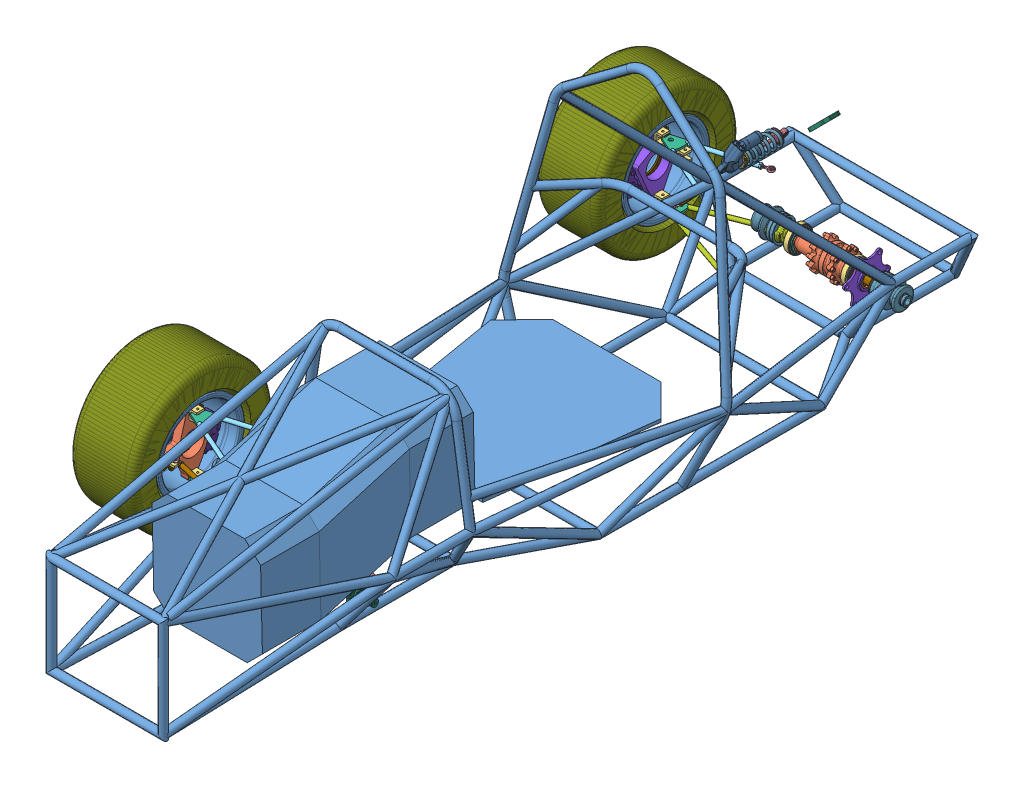
SolidWorks assembly ASSEM_Suspension_RevA, configuration Default. Lengths in mm.
Overall size (1111.1 1095.41 2655.91).
346 component instances, 33 part files, 25 mates.
Components (placement in the parent):
- 2024_Chassis_V1_RevA-1: 2024_Chassis_V1_RevA [Default<As Machined>] at origin size (743.23 992.29 2569.32)
- Differential Assembly-1: Differential Assembly [Default] at (-98.7457 437.9567 -745.2888) x (1 0 0) z (0 -0.960953 -0.276711) size (486.11 199.53 196.01)
  - Drexler Differential-1: Drexler Differential [Default] at (98.7457 177.1174 168.5551) x (0 0.999802 -0.019913) z (0 0.019913 0.999802) size (100 234.25 100)
  - SKF_32010 X-1: SKF_32010 X [Default] at (175.1207 177.1174 168.5551) x (-1 0 0) z (0 -0.454274 -0.890862) size (21.27 80 80)
    - 32010 X_or-1: 32010 X_or [Default] x (1 0 0) z (0 0 -1) size (15.5 80 80)
    - 32010 X_r-1: 32010 X_r [Default] x (1 0 0) z (0 -0.24869 -0.968583) size (15.81 10.45 7.5)
    - 32010 X_r-2: 32010 X_r [Default] x (1 0 0) z (0 -0.481754 -0.876307) size (15.81 10.45 7.5)
    - 32010 X_r-3: 32010 X_r [Default] x (1 0 0) z (0 -0.684547 -0.728969) size (15.81 10.45 7.5)
    - 32010 X_r-4: 32010 X_r [Default] x (1 0 0) z (0 -0.844328 -0.535827) size (15.81 10.45 7.5)
    - 32010 X_r-5: 32010 X_r [Default] x (1 0 0) z (0 -0.951057 -0.309017) size (15.81 10.45 7.5)
    - 32010 X_r-6: 32010 X_r [Default] x (1 0 0) z (0 -0.998027 -0.062791) size (15.81 10.45 7.5)
    - 32010 X_r-7: 32010 X_r [Default] x (1 0 0) z (0 -0.982287 0.187381) size (15.81 10.45 7.5)
    - 32010 X_r-8: 32010 X_r [Default] x (1 0 0) z (0 -0.904827 0.425779) size (15.81 10.45 7.5)
    - 32010 X_r-9: 32010 X_r [Default] x (1 0 0) z (0 -0.770513 0.637424) size (15.81 10.45 7.5)
    - 32010 X_r-10: 32010 X_r [Default] x (1 0 0) z (0 -0.587785 0.809017) size (15.81 10.45 7.5)
    - 32010 X_r-11: 32010 X_r [Default] x (1 0 0) z (0 -0.368125 0.929776) size (15.81 10.45 7.5)
    - 32010 X_r-12: 32010 X_r [Default] x (1 0 0) z (0 -0.125333 0.992115) size (15.81 10.45 7.5)
    - 32010 X_r-13: 32010 X_r [Default] x (1 0 0) z (0 0.125333 0.992115) size (15.81 10.45 7.5)
    - 32010 X_r-14: 32010 X_r [Default] x (1 0 0) z (0 0.368125 0.929776) size (15.81 10.45 7.5)
    - 32010 X_r-15: 32010 X_r [Default] x (1 0 0) z (0 0.587785 0.809017) size (15.81 10.45 7.5)
    - 32010 X_r-16: 32010 X_r [Default] x (1 0 0) z (0 0.770513 0.637424) size (15.81 10.45 7.5)
    - 32010 X_r-17: 32010 X_r [Default] x (1 0 0) z (0 0.904827 0.425779) size (15.81 10.45 7.5)
    - 32010 X_r-18: 32010 X_r [Default] x (1 0 0) z (0 0.982287 0.187381) size (15.81 10.45 7.5)
    - 32010 X_r-19: 32010 X_r [Default] x (1 0 0) z (0 0.998027 -0.062791) size (15.81 10.45 7.5)
    - 32010 X_r-20: 32010 X_r [Default] x (1 0 0) z (0 0.951057 -0.309017) size (15.81 10.45 7.5)
    - 32010 X_r-21: 32010 X_r [Default] x (1 0 0) z (0 0.844328 -0.535827) size (15.81 10.45 7.5)
    - 32010 X_r-22: 32010 X_r [Default] x (1 0 0) z (0 0.684547 -0.728969) size (15.81 10.45 7.5)
    - 32010 X_r-23: 32010 X_r [Default] x (1 0 0) z (0 0.481754 -0.876307) size (15.81 10.45 7.5)
    - 32010 X_r-24: 32010 X_r [Default] x (1 0 0) z (0 0.24869 -0.968583) size (15.81 10.45 7.5)
    - 32010 X_r-25: 32010 X_r [Default] x (1 0 0) z (0 0 -1) size (15.81 10.45 7.5)
    - 32010 X_cage-1: 32010 X_cage [Default] x (1 0 0) z (0 0 -1) size (18.02 76.15 76.15)
    - 32010 X_ir-1: 32010 X_ir [Default] x (1 0 0) z (0 0 -1) size (20 65.95 65.95)
  - SKF_32010 X-2: SKF_32010 X [Default] at (-24.8793 177.1174 168.5551) x (1 0 0) z (0 0.890912 0.454177) size (21.27 80 80)
    - 32010 X_or-1: 32010 X_or [Default] x (1 0 0) z (0 0 -1) size (15.5 80 80)
    - 32010 X_r-1: 32010 X_r [Default] x (1 0 0) z (0 -0.24869 -0.968583) size (15.81 10.45 7.5)
    - 32010 X_r-2: 32010 X_r [Default] x (1 0 0) z (0 -0.481754 -0.876307) size (15.81 10.45 7.5)
    - 32010 X_r-3: 32010 X_r [Default] x (1 0 0) z (0 -0.684547 -0.728969) size (15.81 10.45 7.5)
    - 32010 X_r-4: 32010 X_r [Default] x (1 0 0) z (0 -0.844328 -0.535827) size (15.81 10.45 7.5)
    - 32010 X_r-5: 32010 X_r [Default] x (1 0 0) z (0 -0.951057 -0.309017) size (15.81 10.45 7.5)
    - 32010 X_r-6: 32010 X_r [Default] x (1 0 0) z (0 -0.998027 -0.062791) size (15.81 10.45 7.5)
    - 32010 X_r-7: 32010 X_r [Default] x (1 0 0) z (0 -0.982287 0.187381) size (15.81 10.45 7.5)
    - 32010 X_r-8: 32010 X_r [Default] x (1 0 0) z (0 -0.904827 0.425779) size (15.81 10.45 7.5)
    - 32010 X_r-9: 32010 X_r [Default] x (1 0 0) z (0 -0.770513 0.637424) size (15.81 10.45 7.5)
    - 32010 X_r-10: 32010 X_r [Default] x (1 0 0) z (0 -0.587785 0.809017) size (15.81 10.45 7.5)
    - 32010 X_r-11: 32010 X_r [Default] x (1 0 0) z (0 -0.368125 0.929776) size (15.81 10.45 7.5)
    - 32010 X_r-12: 32010 X_r [Default] x (1 0 0) z (0 -0.125333 0.992115) size (15.81 10.45 7.5)
    - 32010 X_r-13: 32010 X_r [Default] x (1 0 0) z (0 0.125333 0.992115) size (15.81 10.45 7.5)
    - 32010 X_r-14: 32010 X_r [Default] x (1 0 0) z (0 0.368125 0.929776) size (15.81 10.45 7.5)
    - 32010 X_r-15: 32010 X_r [Default] x (1 0 0) z (0 0.587785 0.809017) size (15.81 10.45 7.5)
    - 32010 X_r-16: 32010 X_r [Default] x (1 0 0) z (0 0.770513 0.637424) size (15.81 10.45 7.5)
    - 32010 X_r-17: 32010 X_r [Default] x (1 0 0) z (0 0.904827 0.425779) size (15.81 10.45 7.5)
    - 32010 X_r-18: 32010 X_r [Default] x (1 0 0) z (0 0.982287 0.187381) size (15.81 10.45 7.5)
    - 32010 X_r-19: 32010 X_r [Default] x (1 0 0) z (0 0.998027 -0.062791) size (15.81 10.45 7.5)
    - 32010 X_r-20: 32010 X_r [Default] x (1 0 0) z (0 0.951057 -0.309017) size (15.81 10.45 7.5)
    - 32010 X_r-21: 32010 X_r [Default] x (1 0 0) z (0 0.844328 -0.535827) size (15.81 10.45 7.5)
    - 32010 X_r-22: 32010 X_r [Default] x (1 0 0) z (0 0.684547 -0.728969) size (15.81 10.45 7.5)
    - 32010 X_r-23: 32010 X_r [Default] x (1 0 0) z (0 0.481754 -0.876307) size (15.81 10.45 7.5)
    - 32010 X_r-24: 32010 X_r [Default] x (1 0 0) z (0 0.24869 -0.968583) size (15.81 10.45 7.5)
    - 32010 X_r-25: 32010 X_r [Default] x (1 0 0) z (0 0 -1) size (15.81 10.45 7.5)
    - 32010 X_cage-1: 32010 X_cage [Default] x (1 0 0) z (0 0 -1) size (18.02 76.15 76.15)
    - 32010 X_ir-1: 32010 X_ir [Default] x (1 0 0) z (0 0 -1) size (20 65.95 65.95)
  - D4825 (Drexler Long Tripod Housing)-1: D4825 (Drexler Long Tripod Housing) [Default] at (63.1207 177.1174 168.5551) x (0 0.049326 -0.998783) z (-1 0 0) size (65.36 60.36 166.5)
  - SPIDER_DIFFERENTIAL_ADAPTER-1: SPIDER_DIFFERENTIAL_ADAPTER [Default] at (197.8207 177.0374 168.5892) x (0 -0.59882 0.800884) z (-1 0 0) size (132.58 150 27.1)
  - D4824 (Drexler Medium tripod Housing)-1: D4824 (Drexler Medium tripod Housing) [Default] at (134.3707 177.1174 168.5551) x (0 0.677852 0.735198) z (1 0 0) size (65.36 60.36 155.07)
  - D4672-TA (Tripod)-1: D4672-TA (Tripod) [Default] at (321.1307 160.1151 157.3971) x (1 0 0) z (0 0.676209 0.73671) size (25.48 50.64 55.63)
    - D4672-TA.STEP-1: D4672-TA.STEP [Default] at origin size (25.48 50.64 55.63)
      - FSAE Tripod V2.STEP-1: FSAE Tripod V2.STEP [Default] at (-43.6945 4.946 19.6967) size (24.01 46.11 52.87)
      - FSAE roller_2451.STEP-1: FSAE roller_2451.STEP [Default] at (-43.6945 -7.4365 -1.7504) x (0 0.5 0.866025) z (-1 0 0) size (8.74 25.48 25.48)
      - FSAE roller_2451.STEP-2: FSAE roller_2451.STEP [Default] at (-43.6945 -7.4365 41.1438) x (0 0.5 -0.866025) z (1 0 0) size (8.74 25.48 25.48)
      - FSAE roller_2451.STEP-3: FSAE roller_2451.STEP [Default] at (-43.6945 29.711 19.6967) x (0 -1 0) z (-1 0 0) size (8.74 25.48 25.48)
      - needle.STEP-1: needle.STEP [Default] at (-42.3538 -7.5483 -1.6859) x (1 0 0) z (0 0.5 0.866025) size (1.5 1.5 10.16)
      - needle.STEP-2: needle.STEP [Default] at (-42.3574 -7.2961 -1.8314) x (0.976635 0.186114 -0.107453) z (0 0.5 0.866025) size (1.5 1.5 10.16)
      - needle.STEP-3: needle.STEP [Default] at (-42.4235 -7.0506 -1.9732) x (0.907631 0.363531 -0.209884) z (0 0.5 0.866025) size (1.5 1.5 10.16)
      - needle.STEP-4: needle.STEP [Default] at (-42.5489 -6.823 -2.1046) x (0.796213 0.523959 -0.302508) z (0 0.5 0.866025) size (1.5 1.5 10.16)
      - needle.STEP-5: needle.STEP [Default] at (-42.7279 -6.6242 -2.2194) x (0.647588 0.659903 -0.380995) z (0 0.5 0.866025) size (1.5 1.5 10.16)
      - needle.STEP-6: needle.STEP [Default] at (-42.9521 -6.4632 -2.3123) x (0.468701 0.76501 -0.441678) z (0 0.5 0.866025) size (1.5 1.5 10.16)
      - needle.STEP-7: needle.STEP [Default] at (-43.2109 -6.3478 -2.3789) x (0.267911 0.834367 -0.481722) z (0 0.5 0.866025) size (1.5 1.5 10.16)
      - needle.STEP-8: needle.STEP [Default] at (-43.4924 -6.2833 -2.4162) x (0.054602 0.864733 -0.499254) z (0 0.5 0.866025) size (1.5 1.5 10.16)
      - needle.STEP-9: needle.STEP [Default] at (-43.7833 -6.2726 -2.4224) x (-0.161259 0.854691 -0.493456) z (0 0.5 0.866025) size (1.5 1.5 10.16)
      - needle.STEP-10: needle.STEP [Default] at (-44.07 -6.3163 -2.3971) x (-0.369585 0.804708 -0.464599) z (0 0.5 0.866025) size (1.5 1.5 10.16)
      - needle.STEP-11: needle.STEP [Default] at (-44.3392 -6.4124 -2.3417) x (-0.560639 0.717121 -0.41403) z (0 0.5 0.866025) size (1.5 1.5 10.16)
      - needle.STEP-12: needle.STEP [Default] at (-44.5783 -6.5563 -2.2586) x (-0.725495 0.596023 -0.344114) z (0 0.5 0.866025) size (1.5 1.5 10.16)
      - needle.STEP-13: needle.STEP [Default] at (-44.7761 -6.7413 -2.1517) x (-0.856447 0.447072 -0.258117) z (0 0.5 0.866025) size (1.5 1.5 10.16)
      - needle.STEP-14: needle.STEP [Default] at (-44.9233 -6.9589 -2.0261) x (-0.947378 0.277229 -0.160058) z (0 0.5 0.866025) size (1.5 1.5 10.16)
      - needle.STEP-15: needle.STEP [Default] at (-45.0131 -7.1987 -1.8877) x (-0.994037 0.094432 -0.05452) z (0 0.5 0.866025) size (1.5 1.5 10.16)
      - needle.STEP-16: needle.STEP [Default] at (-45.0413 -7.4497 -1.7428) x (-0.994245 -0.092779 0.053566) z (0 0.5 0.866025) size (1.5 1.5 10.16)
      - needle.STEP-17: needle.STEP [Default] at (-45.0065 -7.7 -1.5982) x (-0.947991 -0.275654 0.159149) z (0 0.5 0.866025) size (1.5 1.5 10.16)
      - needle.STEP-18: needle.STEP [Default] at (-44.9105 -7.9381 -1.4608) x (-0.857437 -0.445647 0.257295) z (0 0.5 0.866025) size (1.5 1.5 10.16)
      - needle.STEP-19: needle.STEP [Default] at (-44.7576 -8.1527 -1.3369) x (-0.726814 -0.594816 0.343417) z (0 0.5 0.866025) size (1.5 1.5 10.16)
      - needle.STEP-20: needle.STEP [Default] at (-44.555 -8.3338 -1.2323) x (-0.562228 -0.716188 0.413491) z (0 0.5 0.866025) size (1.5 1.5 10.16)
      - needle.STEP-21: needle.STEP [Default] at (-44.3122 -8.473 -1.152) x (-0.371368 -0.804092 0.464243) z (0 0.5 0.866025) size (1.5 1.5 10.16)
      - needle.STEP-22: needle.STEP [Default] at (-44.0406 -8.5637 -1.0996) x (-0.163154 -0.854421 0.4933) z (0 0.5 0.866025) size (1.5 1.5 10.16)
      - needle.STEP-23: needle.STEP [Default] at (-43.7528 -8.6018 -1.0776) x (0.052685 -0.864823 0.499306) z (0 0.5 0.866025) size (1.5 1.5 10.16)
      - needle.STEP-24: needle.STEP [Default] at (-43.4622 -8.5854 -1.0871) x (0.266061 -0.834811 0.481978) z (0 0.5 0.866025) size (1.5 1.5 10.16)
      - needle.STEP-25: needle.STEP [Default] at (-43.1825 -8.5153 -1.1275) x (0.467004 -0.765787 0.442128) z (0 0.5 0.866025) size (1.5 1.5 10.16)
      - needle.STEP-26: needle.STEP [Default] at (-42.9268 -8.3949 -1.1971) x (0.646124 -0.660979 0.381616) z (0 0.5 0.866025) size (1.5 1.5 10.16)
      - needle.STEP-27: needle.STEP [Default] at (-42.7069 -8.2296 -1.2925) x (0.79505 -0.525282 0.303272) z (0 0.5 0.866025) size (1.5 1.5 10.16)
      - needle.STEP-28: needle.STEP [Default] at (-42.5332 -8.0272 -1.4093) x (0.906823 -0.365039 0.210755) z (0 0.5 0.866025) size (1.5 1.5 10.16)
      - needle.STEP-29: needle.STEP [Default] at (-42.4137 -7.7973 -1.5421) x (0.97622 -0.187737 0.10839) z (0 0.5 0.866025) size (1.5 1.5 10.16)
      - needle.STEP-30: needle.STEP [Default] at (-42.3538 29.711 19.5676) x (1 0 0) z (0 -1 0) size (1.5 1.5 10.16)
      - needle.STEP-31: needle.STEP [Default] at (-42.3538 -7.3247 41.2084) x (1 0 0) z (0 0.5 -0.866025) size (1.5 1.5 10.16)
      - needle.STEP-32: needle.STEP [Default] at (-42.4137 29.711 19.2801) x (0.97622 0 -0.21678) z (0 -1 0) size (1.5 1.5 10.16)
      - needle.STEP-33: needle.STEP [Default] at (-42.4137 -7.0756 41.3522) x (0.97622 0.187737 0.10839) z (0 0.5 -0.866025) size (1.5 1.5 10.16)
      - needle.STEP-34: needle.STEP [Default] at (-42.5332 29.711 19.0146) x (0.906823 0 -0.421511) z (0 -1 0) size (1.5 1.5 10.16)
      - needle.STEP-35: needle.STEP [Default] at (-42.5332 -6.8457 41.4849) x (0.906823 0.365039 0.210755) z (0 0.5 -0.866025) size (1.5 1.5 10.16)
      - needle.STEP-36: needle.STEP [Default] at (-42.7069 29.711 18.7809) x (0.79505 0 -0.606544) z (0 -1 0) size (1.5 1.5 10.16)
      - needle.STEP-37: needle.STEP [Default] at (-42.7069 -6.6434 41.6017) x (0.79505 0.525282 0.303272) z (0 0.5 -0.866025) size (1.5 1.5 10.16)
      - needle.STEP-38: needle.STEP [Default] at (-42.9268 29.711 18.5901) x (0.646124 0 -0.763232) z (0 -1 0) size (1.5 1.5 10.16)
      - needle.STEP-39: needle.STEP [Default] at (-42.9268 -6.4781 41.6972) x (0.646124 0.660979 0.381616) z (0 0.5 -0.866025) size (1.5 1.5 10.16)
      - needle.STEP-40: needle.STEP [Default] at (-43.1825 29.711 18.4509) x (0.467004 0 -0.884255) z (0 -1 0) size (1.5 1.5 10.16)
      - needle.STEP-41: needle.STEP [Default] at (-43.1825 -6.3576 41.7667) x (0.467004 0.765787 0.442128) z (0 0.5 -0.866025) size (1.5 1.5 10.16)
      - needle.STEP-42: needle.STEP [Default] at (-43.4622 29.711 18.37) x (0.266061 0 -0.963956) z (0 -1 0) size (1.5 1.5 10.16)
      - needle.STEP-43: needle.STEP [Default] at (-43.4622 -6.2875 41.8072) x (0.266061 0.834811 0.481978) z (0 0.5 -0.866025) size (1.5 1.5 10.16)
      - needle.STEP-44: needle.STEP [Default] at (-43.7528 29.711 18.3511) x (0.052685 0 -0.998611) z (0 -1 0) size (1.5 1.5 10.16)
      - needle.STEP-45: needle.STEP [Default] at (-43.7528 -6.2711 41.8166) x (0.052685 0.864823 0.499306) z (0 0.5 -0.866025) size (1.5 1.5 10.16)
      - needle.STEP-46: needle.STEP [Default] at (-44.0406 29.711 18.3951) x (-0.163154 0 -0.986601) z (0 -1 0) size (1.5 1.5 10.16)
      - needle.STEP-47: needle.STEP [Default] at (-44.0406 -6.3092 41.7947) x (-0.163154 0.854421 0.4933) z (0 0.5 -0.866025) size (1.5 1.5 10.16)
      - needle.STEP-48: needle.STEP [Default] at (-44.3122 29.711 18.4999) x (-0.371368 0 -0.928486) z (0 -1 0) size (1.5 1.5 10.16)
      - needle.STEP-49: needle.STEP [Default] at (-44.3122 -6.4 41.7423) x (-0.371368 0.804092 0.464243) z (0 0.5 -0.866025) size (1.5 1.5 10.16)
      - needle.STEP-50: needle.STEP [Default] at (-44.555 29.711 18.6606) x (-0.562228 0 -0.826982) z (0 -1 0) size (1.5 1.5 10.16)
      - needle.STEP-51: needle.STEP [Default] at (-44.555 -6.5392 41.6619) x (-0.562228 0.716188 0.413491) z (0 0.5 -0.866025) size (1.5 1.5 10.16)
      - needle.STEP-52: needle.STEP [Default] at (-44.7576 29.711 18.8697) x (-0.726814 0 -0.686834) z (0 -1 0) size (1.5 1.5 10.16)
      - needle.STEP-53: needle.STEP [Default] at (-44.7576 -6.7203 41.5573) x (-0.726814 0.594816 0.343417) z (0 0.5 -0.866025) size (1.5 1.5 10.16)
      - needle.STEP-54: needle.STEP [Default] at (-44.9105 29.711 19.1175) x (-0.857437 0 -0.514589) z (0 -1 0) size (1.5 1.5 10.16)
      - needle.STEP-55: needle.STEP [Default] at (-44.9105 -6.9349 41.4334) x (-0.857437 0.445647 0.257295) z (0 0.5 -0.866025) size (1.5 1.5 10.16)
      - needle.STEP-56: needle.STEP [Default] at (-45.0065 29.711 19.3924) x (-0.947991 0 -0.318298) z (0 -1 0) size (1.5 1.5 10.16)
      - needle.STEP-57: needle.STEP [Default] at (-45.0065 -7.1729 41.296) x (-0.947991 0.275654 0.159149) z (0 0.5 -0.866025) size (1.5 1.5 10.16)
      - needle.STEP-58: needle.STEP [Default] at (-45.0413 29.711 19.6814) x (-0.994245 0 -0.107132) z (0 -1 0) size (1.5 1.5 10.16)
      - needle.STEP-59: needle.STEP [Default] at (-45.0413 -7.4232 41.1515) x (-0.994245 0.092779 0.053566) z (0 0.5 -0.866025) size (1.5 1.5 10.16)
      - needle.STEP-60: needle.STEP [Default] at (-45.0131 29.711 19.9712) x (-0.994037 0 0.10904) z (0 -1 0) size (1.5 1.5 10.16)
      - needle.STEP-61: needle.STEP [Default] at (-45.0131 -7.6742 41.0066) x (-0.994037 -0.094432 -0.05452) z (0 0.5 -0.866025) size (1.5 1.5 10.16)
      - needle.STEP-62: needle.STEP [Default] at (-44.9233 29.711 20.2482) x (-0.947378 0 0.320117) z (0 -1 0) size (1.5 1.5 10.16)
      - needle.STEP-63: needle.STEP [Default] at (-44.9233 -7.914 40.8681) x (-0.947378 -0.277229 -0.160058) z (0 0.5 -0.866025) size (1.5 1.5 10.16)
      - needle.STEP-64: needle.STEP [Default] at (-44.7761 29.711 20.4994) x (-0.856447 0 0.516234) z (0 -1 0) size (1.5 1.5 10.16)
      - needle.STEP-65: needle.STEP [Default] at (-44.7761 -8.1316 40.7425) x (-0.856447 -0.447072 -0.258117) z (0 0.5 -0.866025) size (1.5 1.5 10.16)
      - needle.STEP-66: needle.STEP [Default] at (-44.5783 29.711 20.7131) x (-0.725495 0 0.688228) z (0 -1 0) size (1.5 1.5 10.16)
      - needle.STEP-67: needle.STEP [Default] at (-44.5783 -8.3166 40.6357) x (-0.725495 -0.596023 -0.344114) z (0 0.5 -0.866025) size (1.5 1.5 10.16)
      - needle.STEP-68: needle.STEP [Default] at (-44.3392 29.711 20.8792) x (-0.560639 0 0.82806) z (0 -1 0) size (1.5 1.5 10.16)
      - needle.STEP-69: needle.STEP [Default] at (-44.3392 -8.4606 40.5526) x (-0.560639 -0.717121 -0.41403) z (0 0.5 -0.866025) size (1.5 1.5 10.16)
      - needle.STEP-70: needle.STEP [Default] at (-44.07 29.711 20.9902) x (-0.369585 0 0.929197) z (0 -1 0) size (1.5 1.5 10.16)
      - needle.STEP-71: needle.STEP [Default] at (-44.07 -8.5566 40.4971) x (-0.369585 -0.804708 -0.464599) z (0 0.5 -0.866025) size (1.5 1.5 10.16)
      - needle.STEP-72: needle.STEP [Default] at (-43.7833 29.711 21.0407) x (-0.161259 0 0.986912) z (0 -1 0) size (1.5 1.5 10.16)
      - needle.STEP-73: needle.STEP [Default] at (-43.7833 -8.6003 40.4719) x (-0.161259 -0.854691 -0.493456) z (0 0.5 -0.866025) size (1.5 1.5 10.16)
      - needle.STEP-74: needle.STEP [Default] at (-43.4924 29.711 21.0283) x (0.054602 0 0.998508) z (0 -1 0) size (1.5 1.5 10.16)
      - needle.STEP-75: needle.STEP [Default] at (-43.4924 -8.5897 40.478) x (0.054602 -0.864733 -0.499254) z (0 0.5 -0.866025) size (1.5 1.5 10.16)
      - needle.STEP-76: needle.STEP [Default] at (-43.2109 29.711 20.9538) x (0.267911 0 0.963444) z (0 -1 0) size (1.5 1.5 10.16)
      - needle.STEP-77: needle.STEP [Default] at (-43.2109 -8.5251 40.5153) x (0.267911 -0.834367 -0.481722) z (0 0.5 -0.866025) size (1.5 1.5 10.16)
      - needle.STEP-78: needle.STEP [Default] at (-42.9521 29.711 20.8205) x (0.468701 0 0.883357) z (0 -1 0) size (1.5 1.5 10.16)
      - needle.STEP-79: needle.STEP [Default] at (-42.9521 -8.4097 40.582) x (0.468701 -0.76501 -0.441678) z (0 0.5 -0.866025) size (1.5 1.5 10.16)
      - needle.STEP-80: needle.STEP [Default] at (-42.7279 29.711 20.6347) x (0.647588 0 0.761991) z (0 -1 0) size (1.5 1.5 10.16)
      - needle.STEP-81: needle.STEP [Default] at (-42.7279 -8.2488 40.6749) x (0.647588 -0.659903 -0.380995) z (0 0.5 -0.866025) size (1.5 1.5 10.16)
      - needle.STEP-82: needle.STEP [Default] at (-42.5489 29.711 20.4051) x (0.796213 0 0.605016) z (0 -1 0) size (1.5 1.5 10.16)
      - needle.STEP-83: needle.STEP [Default] at (-42.5489 -8.0499 40.7897) x (0.796213 -0.523959 -0.302508) z (0 0.5 -0.866025) size (1.5 1.5 10.16)
      - needle.STEP-84: needle.STEP [Default] at (-42.4235 29.711 20.1423) x (0.907631 0 0.419769) z (0 -1 0) size (1.5 1.5 10.16)
      - needle.STEP-85: needle.STEP [Default] at (-42.4235 -7.8224 40.921) x (0.907631 -0.363531 -0.209884) z (0 0.5 -0.866025) size (1.5 1.5 10.16)
      - needle.STEP-86: needle.STEP [Default] at (-42.3574 29.711 19.8588) x (0.976635 0 0.214906) z (0 -1 0) size (1.5 1.5 10.16)
      - needle.STEP-87: needle.STEP [Default] at (-42.3574 -7.5768 41.0628) x (0.976635 -0.186114 -0.107453) z (0 0.5 -0.866025) size (1.5 1.5 10.16)
      - Tripod Retainer.STEP-1: Tripod Retainer.STEP [Default] at (-43.6945 -8.0715 -2.8502) x (0.973299 0.198788 -0.11477) z (0 0.5 0.866025) size (15.88 15.88 1.27)
      - Tripod Retainer.STEP-2: Tripod Retainer.STEP [Default] at (-43.6945 -8.0715 42.2437) x (0.973299 -0.198788 -0.11477) z (0 0.5 -0.866025) size (15.88 15.88 1.27)
      - Tripod Retainer.STEP-3: Tripod Retainer.STEP [Default] at (-43.6945 30.981 19.6967) x (0.973299 0 0.229541) z (0 -1 0) size (15.88 15.88 1.27)
  - D4672-TA (Tripod)-2: D4672-TA (Tripod) [Default] at (-47.6803 161.7899 181.8937) x (1 0 0) z (0 0.890652 -0.454686) size (25.48 50.64 55.63)
    - D4672-TA.STEP-1: D4672-TA.STEP [Default] at origin size (25.48 50.64 55.63)
      - FSAE Tripod V2.STEP-1: FSAE Tripod V2.STEP [Default] at (-43.6945 4.946 19.6967) size (24.01 46.11 52.87)
      - FSAE roller_2451.STEP-1: FSAE roller_2451.STEP [Default] at (-43.6945 -7.4365 -1.7504) x (0 0.5 0.866025) z (-1 0 0) size (8.74 25.48 25.48)
      - FSAE roller_2451.STEP-2: FSAE roller_2451.STEP [Default] at (-43.6945 -7.4365 41.1438) x (0 0.5 -0.866025) z (1 0 0) size (8.74 25.48 25.48)
      - FSAE roller_2451.STEP-3: FSAE roller_2451.STEP [Default] at (-43.6945 29.711 19.6967) x (0 -1 0) z (-1 0 0) size (8.74 25.48 25.48)
      - needle.STEP-1: needle.STEP [Default] at (-42.3538 -7.5483 -1.6859) x (1 0 0) z (0 0.5 0.866025) size (1.5 1.5 10.16)
      - needle.STEP-2: needle.STEP [Default] at (-42.3574 -7.2961 -1.8314) x (0.976635 0.186114 -0.107453) z (0 0.5 0.866025) size (1.5 1.5 10.16)
      - needle.STEP-3: needle.STEP [Default] at (-42.4235 -7.0506 -1.9732) x (0.907631 0.363531 -0.209884) z (0 0.5 0.866025) size (1.5 1.5 10.16)
      - needle.STEP-4: needle.STEP [Default] at (-42.5489 -6.823 -2.1046) x (0.796213 0.523959 -0.302508) z (0 0.5 0.866025) size (1.5 1.5 10.16)
      - needle.STEP-5: needle.STEP [Default] at (-42.7279 -6.6242 -2.2194) x (0.647588 0.659903 -0.380995) z (0 0.5 0.866025) size (1.5 1.5 10.16)
      - needle.STEP-6: needle.STEP [Default] at (-42.9521 -6.4632 -2.3123) x (0.468701 0.76501 -0.441678) z (0 0.5 0.866025) size (1.5 1.5 10.16)
      - needle.STEP-7: needle.STEP [Default] at (-43.2109 -6.3478 -2.3789) x (0.267911 0.834367 -0.481722) z (0 0.5 0.866025) size (1.5 1.5 10.16)
      - needle.STEP-8: needle.STEP [Default] at (-43.4924 -6.2833 -2.4162) x (0.054602 0.864733 -0.499254) z (0 0.5 0.866025) size (1.5 1.5 10.16)
      - needle.STEP-9: needle.STEP [Default] at (-43.7833 -6.2726 -2.4224) x (-0.161259 0.854691 -0.493456) z (0 0.5 0.866025) size (1.5 1.5 10.16)
      - needle.STEP-10: needle.STEP [Default] at (-44.07 -6.3163 -2.3971) x (-0.369585 0.804708 -0.464599) z (0 0.5 0.866025) size (1.5 1.5 10.16)
      - needle.STEP-11: needle.STEP [Default] at (-44.3392 -6.4124 -2.3417) x (-0.560639 0.717121 -0.41403) z (0 0.5 0.866025) size (1.5 1.5 10.16)
      - needle.STEP-12: needle.STEP [Default] at (-44.5783 -6.5563 -2.2586) x (-0.725495 0.596023 -0.344114) z (0 0.5 0.866025) size (1.5 1.5 10.16)
      - needle.STEP-13: needle.STEP [Default] at (-44.7761 -6.7413 -2.1517) x (-0.856447 0.447072 -0.258117) z (0 0.5 0.866025) size (1.5 1.5 10.16)
      - needle.STEP-14: needle.STEP [Default] at (-44.9233 -6.9589 -2.0261) x (-0.947378 0.277229 -0.160058) z (0 0.5 0.866025) size (1.5 1.5 10.16)
      - needle.STEP-15: needle.STEP [Default] at (-45.0131 -7.1987 -1.8877) x (-0.994037 0.094432 -0.05452) z (0 0.5 0.866025) size (1.5 1.5 10.16)
      - needle.STEP-16: needle.STEP [Default] at (-45.0413 -7.4497 -1.7428) x (-0.994245 -0.092779 0.053566) z (0 0.5 0.866025) size (1.5 1.5 10.16)
      - needle.STEP-17: needle.STEP [Default] at (-45.0065 -7.7 -1.5982) x (-0.947991 -0.275654 0.159149) z (0 0.5 0.866025) size (1.5 1.5 10.16)
      - needle.STEP-18: needle.STEP [Default] at (-44.9105 -7.9381 -1.4608) x (-0.857437 -0.445647 0.257295) z (0 0.5 0.866025) size (1.5 1.5 10.16)
      - needle.STEP-19: needle.STEP [Default] at (-44.7576 -8.1527 -1.3369) x (-0.726814 -0.594816 0.343417) z (0 0.5 0.866025) size (1.5 1.5 10.16)
      - needle.STEP-20: needle.STEP [Default] at (-44.555 -8.3338 -1.2323) x (-0.562228 -0.716188 0.413491) z (0 0.5 0.866025) size (1.5 1.5 10.16)
      - needle.STEP-21: needle.STEP [Default] at (-44.3122 -8.473 -1.152) x (-0.371368 -0.804092 0.464243) z (0 0.5 0.866025) size (1.5 1.5 10.16)
      - needle.STEP-22: needle.STEP [Default] at (-44.0406 -8.5637 -1.0996) x (-0.163154 -0.854421 0.4933) z (0 0.5 0.866025) size (1.5 1.5 10.16)
      - needle.STEP-23: needle.STEP [Default] at (-43.7528 -8.6018 -1.0776) x (0.052685 -0.864823 0.499306) z (0 0.5 0.866025) size (1.5 1.5 10.16)
      - needle.STEP-24: needle.STEP [Default] at (-43.4622 -8.5854 -1.0871) x (0.266061 -0.834811 0.481978) z (0 0.5 0.866025) size (1.5 1.5 10.16)
      - needle.STEP-25: needle.STEP [Default] at (-43.1825 -8.5153 -1.1275) x (0.467004 -0.765787 0.442128) z (0 0.5 0.866025) size (1.5 1.5 10.16)
      - needle.STEP-26: needle.STEP [Default] at (-42.9268 -8.3949 -1.1971) x (0.646124 -0.660979 0.381616) z (0 0.5 0.866025) size (1.5 1.5 10.16)
      - needle.STEP-27: needle.STEP [Default] at (-42.7069 -8.2296 -1.2925) x (0.79505 -0.525282 0.303272) z (0 0.5 0.866025) size (1.5 1.5 10.16)
      - needle.STEP-28: needle.STEP [Default] at (-42.5332 -8.0272 -1.4093) x (0.906823 -0.365039 0.210755) z (0 0.5 0.866025) size (1.5 1.5 10.16)
      - needle.STEP-29: needle.STEP [Default] at (-42.4137 -7.7973 -1.5421) x (0.97622 -0.187737 0.10839) z (0 0.5 0.866025) size (1.5 1.5 10.16)
      - needle.STEP-30: needle.STEP [Default] at (-42.3538 29.711 19.5676) x (1 0 0) z (0 -1 0) size (1.5 1.5 10.16)
      - needle.STEP-31: needle.STEP [Default] at (-42.3538 -7.3247 41.2084) x (1 0 0) z (0 0.5 -0.866025) size (1.5 1.5 10.16)
      - needle.STEP-32: needle.STEP [Default] at (-42.4137 29.711 19.2801) x (0.97622 0 -0.21678) z (0 -1 0) size (1.5 1.5 10.16)
      - needle.STEP-33: needle.STEP [Default] at (-42.4137 -7.0756 41.3522) x (0.97622 0.187737 0.10839) z (0 0.5 -0.866025) size (1.5 1.5 10.16)
      - needle.STEP-34: needle.STEP [Default] at (-42.5332 29.711 19.0146) x (0.906823 0 -0.421511) z (0 -1 0) size (1.5 1.5 10.16)
      - needle.STEP-35: needle.STEP [Default] at (-42.5332 -6.8457 41.4849) x (0.906823 0.365039 0.210755) z (0 0.5 -0.866025) size (1.5 1.5 10.16)
      - needle.STEP-36: needle.STEP [Default] at (-42.7069 29.711 18.7809) x (0.79505 0 -0.606544) z (0 -1 0) size (1.5 1.5 10.16)
      - needle.STEP-37: needle.STEP [Default] at (-42.7069 -6.6434 41.6017) x (0.79505 0.525282 0.303272) z (0 0.5 -0.866025) size (1.5 1.5 10.16)
      - needle.STEP-38: needle.STEP [Default] at (-42.9268 29.711 18.5901) x (0.646124 0 -0.763232) z (0 -1 0) size (1.5 1.5 10.16)
      - needle.STEP-39: needle.STEP [Default] at (-42.9268 -6.4781 41.6972) x (0.646124 0.660979 0.381616) z (0 0.5 -0.866025) size (1.5 1.5 10.16)
      - needle.STEP-40: needle.STEP [Default] at (-43.1825 29.711 18.4509) x (0.467004 0 -0.884255) z (0 -1 0) size (1.5 1.5 10.16)
      - needle.STEP-41: needle.STEP [Default] at (-43.1825 -6.3576 41.7667) x (0.467004 0.765787 0.442128) z (0 0.5 -0.866025) size (1.5 1.5 10.16)
      - needle.STEP-42: needle.STEP [Default] at (-43.4622 29.711 18.37) x (0.266061 0 -0.963956) z (0 -1 0) size (1.5 1.5 10.16)
      - needle.STEP-43: needle.STEP [Default] at (-43.4622 -6.2875 41.8072) x (0.266061 0.834811 0.481978) z (0 0.5 -0.866025) size (1.5 1.5 10.16)
      - needle.STEP-44: needle.STEP [Default] at (-43.7528 29.711 18.3511) x (0.052685 0 -0.998611) z (0 -1 0) size (1.5 1.5 10.16)
      - needle.STEP-45: needle.STEP [Default] at (-43.7528 -6.2711 41.8166) x (0.052685 0.864823 0.499306) z (0 0.5 -0.866025) size (1.5 1.5 10.16)
      - needle.STEP-46: needle.STEP [Default] at (-44.0406 29.711 18.3951) x (-0.163154 0 -0.986601) z (0 -1 0) size (1.5 1.5 10.16)
      - needle.STEP-47: needle.STEP [Default] at (-44.0406 -6.3092 41.7947) x (-0.163154 0.854421 0.4933) z (0 0.5 -0.866025) size (1.5 1.5 10.16)
      - needle.STEP-48: needle.STEP [Default] at (-44.3122 29.711 18.4999) x (-0.371368 0 -0.928486) z (0 -1 0) size (1.5 1.5 10.16)
      - needle.STEP-49: needle.STEP [Default] at (-44.3122 -6.4 41.7423) x (-0.371368 0.804092 0.464243) z (0 0.5 -0.866025) size (1.5 1.5 10.16)
      - needle.STEP-50: needle.STEP [Default] at (-44.555 29.711 18.6606) x (-0.562228 0 -0.826982) z (0 -1 0) size (1.5 1.5 10.16)
      - needle.STEP-51: needle.STEP [Default] at (-44.555 -6.5392 41.6619) x (-0.562228 0.716188 0.413491) z (0 0.5 -0.866025) size (1.5 1.5 10.16)
      - needle.STEP-52: needle.STEP [Default] at (-44.7576 29.711 18.8697) x (-0.726814 0 -0.686834) z (0 -1 0) size (1.5 1.5 10.16)
      - needle.STEP-53: needle.STEP [Default] at (-44.7576 -6.7203 41.5573) x (-0.726814 0.594816 0.343417) z (0 0.5 -0.866025) size (1.5 1.5 10.16)
      - needle.STEP-54: needle.STEP [Default] at (-44.9105 29.711 19.1175) x (-0.857437 0 -0.514589) z (0 -1 0) size (1.5 1.5 10.16)
      - needle.STEP-55: needle.STEP [Default] at (-44.9105 -6.9349 41.4334) x (-0.857437 0.445647 0.257295) z (0 0.5 -0.866025) size (1.5 1.5 10.16)
      - needle.STEP-56: needle.STEP [Default] at (-45.0065 29.711 19.3924) x (-0.947991 0 -0.318298) z (0 -1 0) size (1.5 1.5 10.16)
      - needle.STEP-57: needle.STEP [Default] at (-45.0065 -7.1729 41.296) x (-0.947991 0.275654 0.159149) z (0 0.5 -0.866025) size (1.5 1.5 10.16)
      - needle.STEP-58: needle.STEP [Default] at (-45.0413 29.711 19.6814) x (-0.994245 0 -0.107132) z (0 -1 0) size (1.5 1.5 10.16)
      - needle.STEP-59: needle.STEP [Default] at (-45.0413 -7.4232 41.1515) x (-0.994245 0.092779 0.053566) z (0 0.5 -0.866025) size (1.5 1.5 10.16)
      - needle.STEP-60: needle.STEP [Default] at (-45.0131 29.711 19.9712) x (-0.994037 0 0.10904) z (0 -1 0) size (1.5 1.5 10.16)
      - needle.STEP-61: needle.STEP [Default] at (-45.0131 -7.6742 41.0066) x (-0.994037 -0.094432 -0.05452) z (0 0.5 -0.866025) size (1.5 1.5 10.16)
      - needle.STEP-62: needle.STEP [Default] at (-44.9233 29.711 20.2482) x (-0.947378 0 0.320117) z (0 -1 0) size (1.5 1.5 10.16)
      - needle.STEP-63: needle.STEP [Default] at (-44.9233 -7.914 40.8681) x (-0.947378 -0.277229 -0.160058) z (0 0.5 -0.866025) size (1.5 1.5 10.16)
      - needle.STEP-64: needle.STEP [Default] at (-44.7761 29.711 20.4994) x (-0.856447 0 0.516234) z (0 -1 0) size (1.5 1.5 10.16)
      - needle.STEP-65: needle.STEP [Default] at (-44.7761 -8.1316 40.7425) x (-0.856447 -0.447072 -0.258117) z (0 0.5 -0.866025) size (1.5 1.5 10.16)
      - needle.STEP-66: needle.STEP [Default] at (-44.5783 29.711 20.7131) x (-0.725495 0 0.688228) z (0 -1 0) size (1.5 1.5 10.16)
      - needle.STEP-67: needle.STEP [Default] at (-44.5783 -8.3166 40.6357) x (-0.725495 -0.596023 -0.344114) z (0 0.5 -0.866025) size (1.5 1.5 10.16)
      - needle.STEP-68: needle.STEP [Default] at (-44.3392 29.711 20.8792) x (-0.560639 0 0.82806) z (0 -1 0) size (1.5 1.5 10.16)
      - needle.STEP-69: needle.STEP [Default] at (-44.3392 -8.4606 40.5526) x (-0.560639 -0.717121 -0.41403) z (0 0.5 -0.866025) size (1.5 1.5 10.16)
      - needle.STEP-70: needle.STEP [Default] at (-44.07 29.711 20.9902) x (-0.369585 0 0.929197) z (0 -1 0) size (1.5 1.5 10.16)
      - needle.STEP-71: needle.STEP [Default] at (-44.07 -8.5566 40.4971) x (-0.369585 -0.804708 -0.464599) z (0 0.5 -0.866025) size (1.5 1.5 10.16)
      - needle.STEP-72: needle.STEP [Default] at (-43.7833 29.711 21.0407) x (-0.161259 0 0.986912) z (0 -1 0) size (1.5 1.5 10.16)
      - needle.STEP-73: needle.STEP [Default] at (-43.7833 -8.6003 40.4719) x (-0.161259 -0.854691 -0.493456) z (0 0.5 -0.866025) size (1.5 1.5 10.16)
      - needle.STEP-74: needle.STEP [Default] at (-43.4924 29.711 21.0283) x (0.054602 0 0.998508) z (0 -1 0) size (1.5 1.5 10.16)
      - needle.STEP-75: needle.STEP [Default] at (-43.4924 -8.5897 40.478) x (0.054602 -0.864733 -0.499254) z (0 0.5 -0.866025) size (1.5 1.5 10.16)
      - needle.STEP-76: needle.STEP [Default] at (-43.2109 29.711 20.9538) x (0.267911 0 0.963444) z (0 -1 0) size (1.5 1.5 10.16)
      - needle.STEP-77: needle.STEP [Default] at (-43.2109 -8.5251 40.5153) x (0.267911 -0.834367 -0.481722) z (0 0.5 -0.866025) size (1.5 1.5 10.16)
      - needle.STEP-78: needle.STEP [Default] at (-42.9521 29.711 20.8205) x (0.468701 0 0.883357) z (0 -1 0) size (1.5 1.5 10.16)
      - needle.STEP-79: needle.STEP [Default] at (-42.9521 -8.4097 40.582) x (0.468701 -0.76501 -0.441678) z (0 0.5 -0.866025) size (1.5 1.5 10.16)
      - needle.STEP-80: needle.STEP [Default] at (-42.7279 29.711 20.6347) x (0.647588 0 0.761991) z (0 -1 0) size (1.5 1.5 10.16)
      - needle.STEP-81: needle.STEP [Default] at (-42.7279 -8.2488 40.6749) x (0.647588 -0.659903 -0.380995) z (0 0.5 -0.866025) size (1.5 1.5 10.16)
      - needle.STEP-82: needle.STEP [Default] at (-42.5489 29.711 20.4051) x (0.796213 0 0.605016) z (0 -1 0) size (1.5 1.5 10.16)
      - needle.STEP-83: needle.STEP [Default] at (-42.5489 -8.0499 40.7897) x (0.796213 -0.523959 -0.302508) z (0 0.5 -0.866025) size (1.5 1.5 10.16)
      - needle.STEP-84: needle.STEP [Default] at (-42.4235 29.711 20.1423) x (0.907631 0 0.419769) z (0 -1 0) size (1.5 1.5 10.16)
      - needle.STEP-85: needle.STEP [Default] at (-42.4235 -7.8224 40.921) x (0.907631 -0.363531 -0.209884) z (0 0.5 -0.866025) size (1.5 1.5 10.16)
      - needle.STEP-86: needle.STEP [Default] at (-42.3574 29.711 19.8588) x (0.976635 0 0.214906) z (0 -1 0) size (1.5 1.5 10.16)
      - needle.STEP-87: needle.STEP [Default] at (-42.3574 -7.5768 41.0628) x (0.976635 -0.186114 -0.107453) z (0 0.5 -0.866025) size (1.5 1.5 10.16)
      - Tripod Retainer.STEP-1: Tripod Retainer.STEP [Default] at (-43.6945 -8.0715 -2.8502) x (0.973299 0.198788 -0.11477) z (0 0.5 0.866025) size (15.88 15.88 1.27)
      - Tripod Retainer.STEP-2: Tripod Retainer.STEP [Default] at (-43.6945 -8.0715 42.2437) x (0.973299 -0.198788 -0.11477) z (0 0.5 -0.866025) size (15.88 15.88 1.27)
      - Tripod Retainer.STEP-3: Tripod Retainer.STEP [Default] at (-43.6945 30.981 19.6967) x (0.973299 0 0.229541) z (0 -1 0) size (15.88 15.88 1.27)
  - 615-3 (Triangular Tripod Housing Boot)-1: 615-3 (Triangular Tripod Housing Boot) [Default] at (336.0855 177.1174 168.5551) x (0 0.694966 -0.719043) z (1 0 0) size (84.51 84.51 88.49)
  - 615-3 (Triangular Tripod Housing Boot)-2: 615-3 (Triangular Tripod Housing Boot) [Default] at (-150.024 177.1174 168.5551) x (0 -0.881387 -0.472395) z (-1 0 0) size (84.51 84.51 88.49)
- KAZ_Steering_Rack_-_Dumb_Solid-1: KAZ_Steering_Rack_-_Dumb_Solid [Default] at (0 198.8947 1049.6828) x (1 0 0) z (0 1 0) size (386.71 91.39 96.37)
- HoosierTyres_43100Slicks-1: HoosierTyres_43100Slicks [Default] at (-712.47 204.47 902.2716) x (0 -1 0) z (0 0 1) size (459.74 205.74 459.74)
- HoosierTyres_43100Slicks-2: HoosierTyres_43100Slicks [Default] at (-737.87 204.47 -621.7284) x (0 1 0) z (0 0 -1) size (459.74 205.74 459.74)
- ASSEM_Front_WheelUprBrakes-1: ASSEM_Front_WheelUprBrakes [Default] at (-619.125 204.47 902.2716) x (-1 0 0) z (0 0 -1) size (205.74 465.04 465.04)
  - Willwood_Calipers-4: Willwood_Calipers [Default] at (-33.147 7.7199 -7.8202) x (0 0.927952 0.372699) z (1 0 0) size (100.77 53.34 71.25)
  - 7inRotor_Custom-1: 7inRotor_Custom [Default] at (-30.607 0 0) x (0 -0.991825 -0.127604) z (0 0.127604 -0.991825) size (175.34 5.08 177.8)
  - HoosierTyres_43100Slicks-1: HoosierTyres_43100Slicks [Default] at (93.345 0 0) x (0 0.999933 0.011596) z (0 -0.011596 0.999933) size (459.74 205.74 459.74)
  - OZ 10x7 FSAE wheel.stp-1: OZ 10x7 FSAE wheel.stp [Default] at (-9.6203 0 0) x (0 0.669999 -0.742362) z (1 0 0) size (282.17 282.17 189.8)
  - Upright_front-2: Upright_front [Default] at (-51.816 0 0) x (0 0 1) z (-1 0 0) size (170.28 202.6 25.4)
  - UBracket_Upright-1: UBracket_Upright [Default] at (-77.216 71.843 -12.7) x (0 1 0) z (1 0 0) size (31.64 25.4 25.4)
  - UBracket_Upright-2: UBracket_Upright [Default] at (-77.216 -105.3614 -12.7) x (0 1 0) z (1 0 0) size (31.64 25.4 25.4)
  - UBracket_Upright-3: UBracket_Upright [Default] at (-77.216 -15.8222 -84.5631) x (0 1 0) z (1 0 0) size (31.64 25.4 25.4)
- Wishbone_Full-2: Wishbone_Full [Default] at (-559.1993 294.0993 900.1762) x (0.063338 0 -0.997992) z (0.997992 0 0.063338) size (221.1 13.97 268.6)
  - Arm_Weldment1-1: Arm_Weldment1 [Default] at (-39.2885 1.138 55.188) x (-0.939693 0 -0.34202) z (0 1 0) size (19.05 229.31 13.97)
    - 60645K121_Ball Joint Rod End-1: 60645K121_Ball Joint Rod End [60645K121] at (-18.0437 209.4907 -1.138) size (19.05 49.39 9.53)
    - Rod_Wishbone-1: Rod_Wishbone [Default] at (-18.0437 3.9907 -1.138) size (15.98 195.5 13.97)
  - Arm_Weldment1-2: Arm_Weldment1 [Default] at (4.3238 1.138 64.6358) x (-0.939693 0 0.34202) z (0 1 0) size (19.05 229.31 13.97)
    - 60645K121_Ball Joint Rod End-1: 60645K121_Ball Joint Rod End [60645K121] at (-18.0437 209.4907 -1.138) size (19.05 49.39 9.53)
    - Rod_Wishbone-1: Rod_Wishbone [Default] at (-18.0437 3.9907 -1.138) size (15.98 195.5 13.97)
  - Wishbone_Weldment2-1: Wishbone_Weldment2 [Default] at (0.0094 -3.175 33.2314) size (60.81 6.35 56.08)
- FR_Wishbone_Full-1: FR_Wishbone_Full [Default] at (-559.2596 113.415 902.8921) x (-0.018388 0 -0.999831) z (0.999831 0 -0.018388) size (283.72 21.98 364.08)
  - Wishbone_Weldment2-1: Wishbone_Weldment2 [Default] at (0.0094 -3.175 33.2314) size (60.81 6.35 56.08)
  - FR_BottomArm_Weldment1-1: FR_BottomArm_Weldment1 [Default] at (-10.6928 6.9131 82.8687) x (0.794652 0.533737 0.28923) z (0.501549 -0.845651 0.182549) size (19.05 313.21 13.97)
    - 60645K121_Ball Joint Rod End-1: 60645K121_Ball Joint Rod End [60645K121] at (-19.1608 277.8138 -3.9185) size (19.05 49.39 9.53)
    - Rod_Wishbone_B-1: Rod_Wishbone_B [Default] at (-19.1608 -11.5862 -3.9185) size (15.98 284.4 13.97)
  - FR_BottomArm_Weldment1-2: FR_BottomArm_Weldment1 [Default] at (43.952 -9.5492 70.8548) x (0.895366 -0.303509 -0.325887) z (-0.285205 -0.952829 0.103806) size (19.05 313.21 13.97)
    - 60645K121_Ball Joint Rod End-1: 60645K121_Ball Joint Rod End [60645K121] at (-19.1608 277.8138 -3.9185) size (19.05 49.39 9.53)
    - Rod_Wishbone_B-1: Rod_Wishbone_B [Default] at (-19.1608 -11.5862 -3.9185) size (15.98 284.4 13.97)
- ASSEM_Rear_WheelUprBrakes-1: ASSEM_Rear_WheelUprBrakes [Default] at (-644.525 204.47 -621.7284) x (-1 0 0) z (0 0 -1) size (205.74 465.04 465.04)
  - Willwood_Calipers-4: Willwood_Calipers [Default] at (-33.147 7.7179 7.821) x (0 -0.927953 0.372696) z (1 0 0) size (100.77 53.34 71.25)
  - 7inRotor_Custom-1: 7inRotor_Custom [Default] at (-30.607 0 0) x (0 -0.991825 -0.127604) z (0 0.127604 -0.991825) size (175.34 5.08 177.8)
  - HoosierTyres_43100Slicks-1: HoosierTyres_43100Slicks [Default] at (93.345 0 0) x (0 0.999933 0.011596) z (0 -0.011596 0.999933) size (459.74 205.74 459.74)
  - OZ 10x7 FSAE wheel.stp-1: OZ 10x7 FSAE wheel.stp [Default] at (-9.6203 0 0) x (0 0.669999 -0.742362) z (1 0 0) size (282.17 282.17 189.8)
  - UBracket_Upright-1: UBracket_Upright [Default] at (-77.216 71.843 -12.7) x (0 1 0) z (1 0 0) size (31.64 25.4 25.4)
  - UBracket_Upright-2: UBracket_Upright [Default] at (-77.216 -105.3614 -12.7) x (0 1 0) z (1 0 0) size (31.64 25.4 25.4)
  - UBracket_Upright-3: UBracket_Upright [Default] at (-77.216 -15.8222 59.1631) x (0 1 0) z (1 0 0) size (31.64 25.4 25.4)
  - Upright_Rear-2: Upright_Rear [Default] at (-77.216 0 0) x (0 0 -1) z (1 0 0) size (170.28 202.6 25.4)
- FR_Wishbone_Full-2: FR_Wishbone_Full [Default] at (-559.2596 113.415 -621.1079) x (-0.018388 0 -0.999831) z (0.999831 0 -0.018388) size (283.72 21.98 364.08)
  - Wishbone_Weldment2-1: Wishbone_Weldment2 [Default] at (0.0094 -3.175 33.2314) size (60.81 6.35 56.08)
  - FR_BottomArm_Weldment1-1: FR_BottomArm_Weldment1 [Default] at (-10.6928 6.9131 82.8687) x (0.794652 0.533737 0.28923) z (0.501549 -0.845651 0.182549) size (19.05 313.21 13.97)
    - 60645K121_Ball Joint Rod End-1: 60645K121_Ball Joint Rod End [60645K121] at (-19.1608 277.8138 -3.9185) size (19.05 49.39 9.53)
    - Rod_Wishbone_B-1: Rod_Wishbone_B [Default] at (-19.1608 -11.5862 -3.9185) size (15.98 284.4 13.97)
  - FR_BottomArm_Weldment1-2: FR_BottomArm_Weldment1 [Default] at (43.952 -9.5492 70.8548) x (0.895366 -0.303509 -0.325887) z (-0.285205 -0.952829 0.103806) size (19.05 313.21 13.97)
    - 60645K121_Ball Joint Rod End-1: 60645K121_Ball Joint Rod End [60645K121] at (-19.1608 277.8138 -3.9185) size (19.05 49.39 9.53)
    - Rod_Wishbone_B-1: Rod_Wishbone_B [Default] at (-19.1608 -11.5862 -3.9185) size (15.98 284.4 13.97)
- Wishbone_Full-3: Wishbone_Full [Default] at (-559.1993 294.0993 -623.8238) x (0.063338 0 -0.997992) z (0.997992 0 0.063338) size (221.1 13.97 268.6)
  - Arm_Weldment1-1: Arm_Weldment1 [Default] at (-39.2885 1.138 55.188) x (-0.939693 0 -0.34202) z (0 1 0) size (19.05 229.31 13.97)
    - 60645K121_Ball Joint Rod End-1: 60645K121_Ball Joint Rod End [60645K121] at (-18.0437 209.4907 -1.138) size (19.05 49.39 9.53)
    - Rod_Wishbone-1: Rod_Wishbone [Default] at (-18.0437 3.9907 -1.138) size (15.98 195.5 13.97)
  - Arm_Weldment1-2: Arm_Weldment1 [Default] at (4.3238 1.138 64.6358) x (-0.939693 0 0.34202) z (0 1 0) size (19.05 229.31 13.97)
    - 60645K121_Ball Joint Rod End-1: 60645K121_Ball Joint Rod End [60645K121] at (-18.0437 209.4907 -1.138) size (19.05 49.39 9.53)
    - Rod_Wishbone-1: Rod_Wishbone [Default] at (-18.0437 3.9907 -1.138) size (15.98 195.5 13.97)
  - Wishbone_Weldment2-1: Wishbone_Weldment2 [Default] at (0.0094 -3.175 33.2314) size (60.81 6.35 56.08)
- TieRod-1: TieRod [Default] at (-343.9724 201.6783 1005.1556) x (0.223812 0 -0.974632) z (0 1 0) size (19.05 382.22 13.97)
  - RodTubing-1: RodTubing [Default] at (-10.5136 -149.457 1.85) size (15.98 314.8 13.97)
  - 60645K121_Ball Joint Rod End-1: 60645K121_Ball Joint Rod End [60645K121] at (-10.5136 170.0984 1.85) size (19.05 49.39 9.53)
  - 60645K121_Ball Joint Rod End-2: 60645K121_Ball Joint Rod End [60645K121] at (-10.5136 -164.5 1.85) x (-1 0 0) z (0 0 1) size (19.05 49.39 9.53)
- Ohlins TTX25 Shock 50mm-1: Ohlins TTX25 Shock 50mm [Default] at (-302.3187 305.8561 941.9451) x (0.651974 -0.755599 -0.063248) z (-0.063248 -0.137317 0.988506) size (68.2 222.5 95.1)
  - Body-1: Body [Default] at origin size (40.15 132 80.5)
  - M8 ball-1: M8 ball [Default] x (0 0 -1) z (1 0 0) size (12.5 12.5 8)
  - M8 ball-2: M8 ball [Default] at (0 -199.5 0) x (0 0 -1) z (1 0 0) size (12.5 12.5 8)
  - Tightening nut-1: Tightening nut [Default] at (0 -4 0) x (-0.593403 0 0.804906) z (-0.804906 0 -0.593403) size (48.77 20 48.77)
  - Piston-1: Piston [Default] at (0 0.13 0) x (-0.999632 0 -0.027131) z (0.027131 0 -0.999632) size (46 115.5 45.56)
  - Spring-1: Spring [Default] at (0 -176 0) size (54.68 133 54.06)
- Rocker-1: Rocker [Default] at (-147.5 187.7104 976.6436) x (0.804613 0.5938 0) z (0.5938 -0.804613 0) size (63.62 10 93.34)
- Ohlins TTX25 Shock 50mm-2: Ohlins TTX25 Shock 50mm [Default] at (-99.1058 217.885 964.6775) x (0.032629 0.170283 -0.984855) z (0.185343 0.967258 0.173381) size (68.2 222.5 95.1)
  - Body-1: Body [Default] at origin size (40.15 132 80.5)
  - M8 ball-1: M8 ball [Default] x (0 0 -1) z (1 0 0) size (12.5 12.5 8)
  - M8 ball-2: M8 ball [Default] at (0 -199.5 0) x (0 0 -1) z (1 0 0) size (12.5 12.5 8)
  - Tightening nut-1: Tightening nut [Default] at (0 -4 0) x (-0.593403 0 0.804906) z (-0.804906 0 -0.593403) size (48.77 20 48.77)
  - Piston-1: Piston [Default] at (0 0.13 0) x (-0.999632 0 -0.027131) z (0.027131 0 -0.999632) size (46 115.5 45.56)
  - Spring-1: Spring [Default] at (0 -176 0) size (54.68 133 54.06)
- TieRod-2: TieRod [Default] at (-357.0703 188.7781 936.8582) x (-0.314168 0.923729 -0.21914) z (-0.286049 0.127996 0.949628) size (19.05 382.22 13.97)
  - RodTubing-1: RodTubing [Default] at (-10.5136 -149.457 1.85) size (15.98 314.8 13.97)
  - 60645K121_Ball Joint Rod End-1: 60645K121_Ball Joint Rod End [60645K121] at (-10.5136 170.0984 1.85) size (19.05 49.39 9.53)
  - 60645K121_Ball Joint Rod End-2: 60645K121_Ball Joint Rod End [60645K121] at (-10.5136 -164.5 1.85) x (-1 0 0) z (0 0 1) size (19.05 49.39 9.53)
- Ohlins TTX25 Shock 50mm-3: Ohlins TTX25 Shock 50mm [Default] at (-272.5 387.5522 -532.5885) x (-0.956418 0.292 0) z (0.292 0.956418 0) size (68.2 222.5 95.1)
  - Body-1: Body [Default] at origin size (40.15 132 80.5)
  - M8 ball-1: M8 ball [Default] x (0 0 -1) z (1 0 0) size (12.5 12.5 8)
  - M8 ball-2: M8 ball [Default] at (0 -199.5 0) x (0 0 -1) z (1 0 0) size (12.5 12.5 8)
  - Tightening nut-1: Tightening nut [Default] at (0 -4 0) x (-0.593403 0 0.804906) z (-0.804906 0 -0.593403) size (48.77 20 48.77)
  - Piston-1: Piston [Default] at (0 0.13 0) x (-0.999632 0 -0.027131) z (0.027131 0 -0.999632) size (46 115.5 45.56)
  - Spring-1: Spring [Default] at (0 -176 0) size (54.68 133 54.06)
- Rocker-2: Rocker [Default] at (-283.8731 336.108 -843.5758) x (0.707107 0.707107 0.000349) z (0.000349 -0.000843 1) size (63.62 10 93.34)
- TieRod-3: TieRod [Default] at (-414.5377 241.6796 -687.0529) x (-0.767759 0.434558 -0.470856) z (0.172625 -0.567406 -0.80514) size (19.05 382.22 13.97)
  - RodTubing-1: RodTubing [Default] at (-10.5136 -149.457 1.85) size (15.98 314.8 13.97)
  - 60645K121_Ball Joint Rod End-1: 60645K121_Ball Joint Rod End [60645K121] at (-10.5136 170.0984 1.85) size (19.05 49.39 9.53)
  - 60645K121_Ball Joint Rod End-2: 60645K121_Ball Joint Rod End [60645K121] at (-10.5136 -164.5 1.85) x (-1 0 0) z (0 0 1) size (19.05 49.39 9.53)
Mates (geometry in assembly coordinates):
- Concentric1: concentric anti-aligned: cylinder of Differential Assembly-1/Drexler Differential-1 through (-121.625 226.9728 -621.7284) axis (1 0 0) radius 25
- Coincident2: coincident: unknown of Differential Assembly-1/Drexler Differential-1
- Coincident4: coincident anti-aligned: plane of KAZ_Steering_Rack_-_Dumb_Solid-1 through (139.7 173.4947 1079.6167) normal (0 -1 0)
- Coincident5: coincident anti-aligned: plane of KAZ_Steering_Rack_-_Dumb_Solid-1 through (0 198.8947 1049.6828) normal (-1 0 0)
- Tangent1: tangent anti-aligned: cylinder of HoosierTyres_43100Slicks-1 through (-712.47 204.47 902.2716) axis (-1 0 0) radius 229.87
- Tangent2: tangent anti-aligned: cylinder of HoosierTyres_43100Slicks-2 through (-737.87 204.47 -621.7284) axis (-1 0 0) radius 229.87
- Distance1: distance = 25.4 mm aligned: plane of HoosierTyres_43100Slicks-1 through (-506.73 356.87 902.2716) normal (1 0 0); plane of HoosierTyres_43100Slicks-2 through (-532.13 52.07 -621.7284) normal (1 0 0)
- Coincident8: coincident anti-aligned: plane of HoosierTyres_43100Slicks-1 through (-712.47 204.47 902.2716) normal (0 0 1)
- Coincident9: coincident aligned: plane of HoosierTyres_43100Slicks-2 through (-737.87 204.47 -621.7284) normal (0 0 -1)
- Distance3: distance = 609.6 mm anti-aligned: plane of HoosierTyres_43100Slicks-1 through (-609.6 204.47 902.2716) normal (-1 0 0)
- Concentric2: concentric aligned: cylinder of HoosierTyres_43100Slicks-1 through (-712.47 204.47 902.2716) axis (-1 0 0) radius 229.87; cylinder of ASSEM_HubWBrakes-1/HoosierTyres_43100Slicks-1 through (-712.47 204.47 902.2716) axis (-1 0 0) radius 229.87
- Coincident10: coincident aligned: plane of HoosierTyres_43100Slicks-1 through (-712.47 356.87 902.2716) normal (-1 0 0); plane of ASSEM_HubWBrakes-1/HoosierTyres_43100Slicks-1 through (-712.47 52.0802 904.0388) normal (-1 0 0)
- Parallel2: parallel anti-aligned: plane of ASSEM_HubWBrakes-1/Upright_front-2 through (-567.309 204.47 902.2716) normal (0 0 -1)
- Concentric4: concentric anti-aligned: cylinder of ASSEM_HubWBrakes-1/UBracket_Upright-1 through (-526.034 276.313 902.2716) axis (0 1 0) radius 3.302; cylinder of Wishbone_Full-2/Wishbone_Weldment2-1 through (-526.034 297.2743 902.2716) axis (0 -1 0) radius 6.35
- Concentric7: concentric aligned: circle of ASSEM_HubWBrakes-1/UBracket_Upright-2; cylinder of FR_Wishbone_Full-1/Wishbone_Weldment2-1 through (-526.034 116.59 902.2716) axis (0 -1 0) radius 6.35
- Concentric8: concentric aligned: cylinder of HoosierTyres_43100Slicks-2 through (-737.87 204.47 -621.7284) axis (-1 0 0) radius 152.4; cylinder of ASSEM_Rear_WheelUprBrakes-1/HoosierTyres_43100Slicks-1 through (-737.87 204.47 -621.7284) axis (-1 0 0) radius 229.87
- Coincident11: coincident aligned: plane of HoosierTyres_43100Slicks-2 through (-532.13 52.07 -621.7284) normal (1 0 0); plane of ASSEM_Rear_WheelUprBrakes-1/HoosierTyres_43100Slicks-1 through (-532.13 52.0802 -619.9612) normal (1 0 0)
- Concentric9: concentric anti-aligned: circle of ASSEM_Front_WheelUprBrakes-1/UBracket_Upright-3; cylinder of TieRod-1/60645K121_Ball Joint Rod End-1 through (-526.034 198.7658 974.1348) axis (0 1 0) radius 3.175
- Parallel3: parallel aligned: line of Ohlins TTX25 Shock 50mm-1 through (-393.0661 228.9346 925.4533) axis (0.755599 0.640479 0.137317)
- Concentric10: concentric aligned: cylinder of Rocker-1 through (-147.5 187.7104 986.6436) axis (0 0 -1) radius 10.5879
- Coincident12: coincident anti-aligned: line of Ohlins TTX25 Shock 50mm-2 through (18.8483 195.283 964.6775) axis (-0.982132 0.188193 0)
- Concentric11: concentric anti-aligned: cylinder of TieRod-2/RodTubing-1 through (-494.9204 123.22 906.1191) axis (0.905248 0.361028 0.22402) radius 6.35
- Coincident13: coincident aligned: line of Ohlins TTX25 Shock 50mm-3 through (-272.5 387.5522 -652.6885) axis (0 0 1)
- Coincident15: coincident aligned: plane of Rocker-2 through (-283.8731 336.108 -843.5758) normal (0.707107 -0.707106 -0.000843)
- Concentric12: concentric anti-aligned: cylinder of TieRod-3/RodTubing-1 through (-310.2925 344.7136 -739.6111) axis (-0.617046 -0.699435 0.360616) radius 6.35
